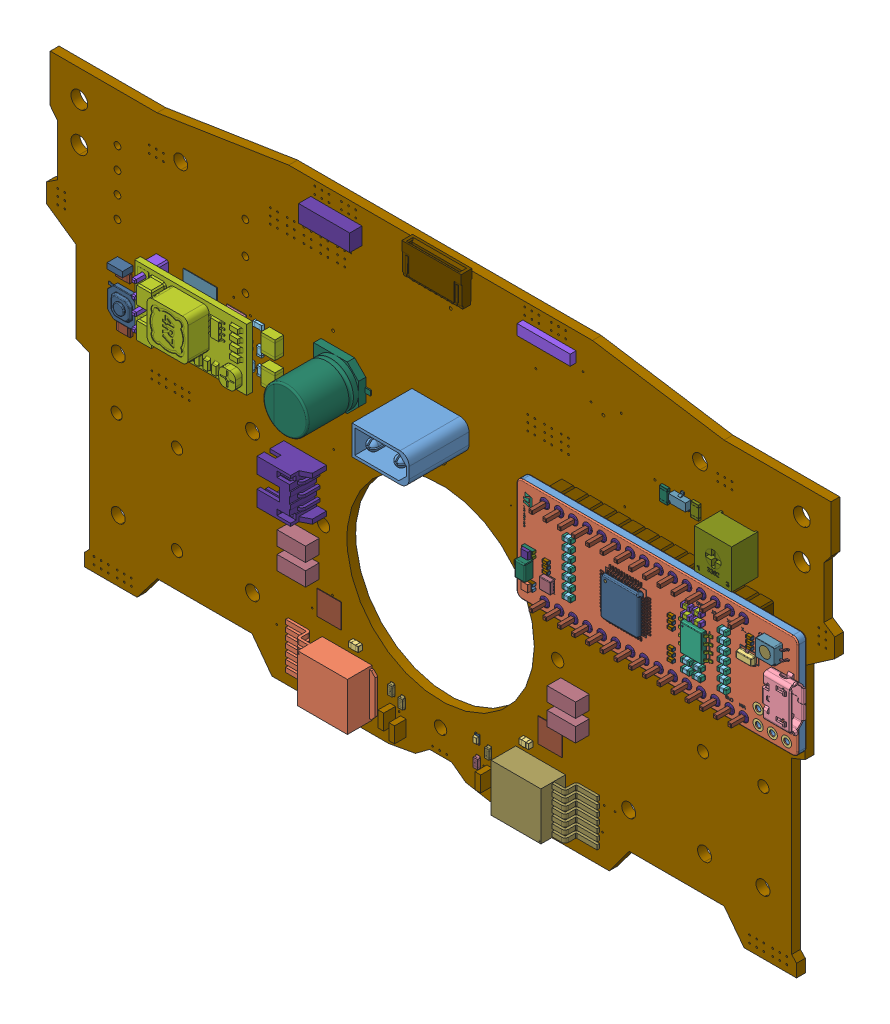
SolidWorks assembly placa v11, configuration Predeterminado. Lengths in mm.
Overall size (140.86 80.97 16.6).
216 component instances, 71 part files, 0 mates.
Components (placement in the parent):
- placa v11.step-1: placa v11.step [Predeterminado] at origin size (140.86 80.97 16.6)
  - PCB Component.step-1: PCB Component.step [Predeterminado] at origin size (140.86 80.97 16.6)
    - LED-0603 (1).step-1: LED-0603 (1).step [Predeterminado] at (70.275 8.61 1.57) x (0 -1 0) z (0 0 1) size (1.61 0.81 0.61)
      - Pocket002.step-1: Pocket002.step [Predeterminado] at origin size (0.41 0.81 0.21)
      - Pad004.step-1: Pad004.step [Predeterminado] x (1 0 0) z (0 0 -1) size (0.4 0.8 0)
      - Fillet.step-1: Fillet.step [Predeterminado] at origin size (1 0.7 0.4)
      - Pocket001.step-1: Pocket001.step [Predeterminado] at origin size (0.4 0.8 0.2)
      - Pad.step-1: Pad.step [Predeterminado] at origin size (0.8 0.8 0.2)
    - ARDUINO-NANO-3.0.step-1: ARDUINO-NANO-3.0.step [Predeterminado] at (104.204 47.47 1.57) size (51.66 18.54 11.82)
      - 1.step.step-1: 1.step.step [Predeterminado] at (9.2423 0.0433 4.14) x (0 -1 0) z (0 0 1) size (4.9 6 1)
        - 1-0.step.step-1: 1-0.step.step [Predeterminado] at (0 0 0.08) size (4.9 3.9 0.92)
        - 2.step.step-1: 2.step.step [Predeterminado] at (0.635 0 0) size (4.23 6 0.62)
        - Name1.step.step-1: Name1.step.step [Predeterminado] at (-0.0045 -0.5756 0.3787) x (-1 0 0) z (0 1 0) size (0.25 0.13 0.25)
        - thermal pad.step.step-1: thermal pad.step.step [Predeterminado] at (0 0 0.08) x (-1 0 0) z (0 0 -1) size (3.2 2.4 0.1)
      - QFP Template.step.step-1: QFP Template.step.step [Predeterminado] at (-3.3256 -0.4727 4.14) x (0 -1 0) z (0 0 1) size (9 9 1.2)
        - Body.step.step-1: Body.step.step [Predeterminado] at (0 0 0.15) size (7 7 1.05)
        - Leg.step.step-1: Leg.step.step [Predeterminado] at (0 0.25 0) x (1 0 0) z (0 -1 0) size (9 0.75 5.72)
        - Leg.step.step-2: Leg.step.step [Predeterminado] at (-0.25 0 0) x (0 1 0) z (1 0 0) size (9 0.75 5.72)
        - name2.step.step-1: name2.step.step [Predeterminado] at (1.2257 1.5908 1.101) size (0.47 0.47 0.1)
      - QFP Template.step (1).step-1: QFP Template.step (1).step [Predeterminado] at (11.7079 0.2587 2.54) x (0 -1 0) z (0 0 -1) size (9 9 1.2)
        - Body.step.step-1: Body.step.step [Predeterminado] at (0 0 0.15) size (7 7 1.05)
        - Leg.step.step-1: Leg.step.step [Predeterminado] at (0 0.25 0) x (1 0 0) z (0 -1 0) size (9 0.75 5.72)
        - Leg.step.step-2: Leg.step.step [Predeterminado] at (-0.25 0 0) x (0 1 0) z (1 0 0) size (9 0.75 5.72)
        - name2.step.step-1: name2.step.step [Predeterminado] at (1.2257 1.5908 1.101) size (0.47 0.47 0.1)
      - 1-1.step.step-1: 1-1.step.step [Predeterminado] at (-17.0798 -4.3486 4.14) size (2 2 0.8)
        - 1-2.step.step-1: 1-2.step.step [Predeterminado] at (0 0 0.02) size (2 2 0.78)
        - 2-3.step.step-1: 2-3.step.step [Predeterminado] at origin size (2 1.6 0.2)
      - 1-2-4.step.step-1: 1-2-4.step.step [Predeterminado] at (-20.4345 -1.0096 4.14) size (2 1.25 1.09)
        - 1-5.step.step-1: 1-5.step.step [Predeterminado] at (0 0 0.01) size (1.98 1.25 0.58)
        - 2-6.step.step-1: 2-6.step.step [Predeterminado] at (0.001 0 0) size (2 1.25 0.6)
        - 3.step.step-1: 3.step.step [Predeterminado] at (0.001 0 0.59) x (-1 0 0) z (0 0 1) size (1.45 1.25 0.5)
      - 1-3.step.step-1: 1-3.step.step [Predeterminado] at (-20.4345 -6.0538 4.14) size (2 1.25 1.09)
        - 1-7.step.step-1: 1-7.step.step [Predeterminado] at (0 0 0.01) size (1.98 1.25 0.58)
        - 2-8.step.step-1: 2-8.step.step [Predeterminado] at (0.001 0 0) size (2 1.25 0.6)
        - 3-9.step.step-1: 3-9.step.step [Predeterminado] at (0.001 0 0.59) x (-1 0 0) z (0 0 1) size (1.45 1.25 0.5)
      - 1-4.step.step-1: 1-4.step.step [Predeterminado] at (18.758 2.4348 4.14) x (0 -1 0) z (0 0 1) size (2.3 2.86 1.1)
        - 1-10.step.step-1: 1-10.step.step [Predeterminado] at (0 0 0.055) size (1.3 2.86 1.04)
        - 2-11.step.step-1: 2-11.step.step [Predeterminado] x (1 0 0) z (0 -1 0) size (2.3 0.55 2.35)
      - 3-12.step.step-1: 3-12.step.step [Predeterminado] at (14.649 -4.6077 5.09) x (-1 0 0) z (0 0 -1) size (1.6 0.8 0.95)
        - 1-13.step.step-1: 1-13.step.step [Predeterminado] at (-0.78 0.38 0.93) x (1 0 0) z (0 0 -1) size (1.56 0.76 0.91)
        - 2-14.step.step-1: 2-14.step.step [Predeterminado] at (0 0 0.95) x (1 0 0) z (0 0 -1) size (1.6 0.8 0.95)
      - 3-12.step (1).step-1: 3-12.step (1).step [Predeterminado] at (-13.1027 -4.224 5.09) x (-1 0 0) z (0 0 -1) size (1.6 0.8 0.95)
        - 1-13.step.step-1: 1-13.step.step [Predeterminado] at (-0.78 0.38 0.93) x (1 0 0) z (0 0 -1) size (1.56 0.76 0.91)
        - 2-14.step.step-1: 2-14.step.step [Predeterminado] at (0 0 0.95) x (1 0 0) z (0 0 -1) size (1.6 0.8 0.95)
      - 3-12.step (2).step-1: 3-12.step (2).step [Predeterminado] at (14.649 -3.1077 5.09) x (-1 0 0) z (0 0 -1) size (1.6 0.8 0.95)
        - 1-13.step.step-1: 1-13.step.step [Predeterminado] at (-0.78 0.38 0.93) x (1 0 0) z (0 0 -1) size (1.56 0.76 0.91)
        - 2-14.step.step-1: 2-14.step.step [Predeterminado] at (0 0 0.95) x (1 0 0) z (0 0 -1) size (1.6 0.8 0.95)
      - 3-12.step (3).step-1: 3-12.step (3).step [Predeterminado] at (-13.1027 -2.724 5.09) x (-1 0 0) z (0 0 -1) size (1.6 0.8 0.95)
        - 1-13.step.step-1: 1-13.step.step [Predeterminado] at (-0.78 0.38 0.93) x (1 0 0) z (0 0 -1) size (1.56 0.76 0.91)
        - 2-14.step.step-1: 2-14.step.step [Predeterminado] at (0 0 0.95) x (1 0 0) z (0 0 -1) size (1.6 0.8 0.95)
      - 3-12.step (4).step-1: 3-12.step (4).step [Predeterminado] at (14.649 -1.6077 5.09) x (-1 0 0) z (0 0 -1) size (1.6 0.8 0.95)
        - 1-13.step.step-1: 1-13.step.step [Predeterminado] at (-0.78 0.38 0.93) x (1 0 0) z (0 0 -1) size (1.56 0.76 0.91)
        - 2-14.step.step-1: 2-14.step.step [Predeterminado] at (0 0 0.95) x (1 0 0) z (0 0 -1) size (1.6 0.8 0.95)
      - 3-12.step (5).step-1: 3-12.step (5).step [Predeterminado] at (-13.1027 -1.224 5.09) x (-1 0 0) z (0 0 -1) size (1.6 0.8 0.95)
        - 1-13.step.step-1: 1-13.step.step [Predeterminado] at (-0.78 0.38 0.93) x (1 0 0) z (0 0 -1) size (1.56 0.76 0.91)
        - 2-14.step.step-1: 2-14.step.step [Predeterminado] at (0 0 0.95) x (1 0 0) z (0 0 -1) size (1.6 0.8 0.95)
      - 3-12.step (6).step-1: 3-12.step (6).step [Predeterminado] at (14.649 -0.1077 5.09) x (-1 0 0) z (0 0 -1) size (1.6 0.8 0.95)
        - 1-13.step.step-1: 1-13.step.step [Predeterminado] at (-0.78 0.38 0.93) x (1 0 0) z (0 0 -1) size (1.56 0.76 0.91)
        - 2-14.step.step-1: 2-14.step.step [Predeterminado] at (0 0 0.95) x (1 0 0) z (0 0 -1) size (1.6 0.8 0.95)
      - 3-12.step (7).step-1: 3-12.step (7).step [Predeterminado] at (-13.1027 0.276 5.09) x (-1 0 0) z (0 0 -1) size (1.6 0.8 0.95)
        - 1-13.step.step-1: 1-13.step.step [Predeterminado] at (-0.78 0.38 0.93) x (1 0 0) z (0 0 -1) size (1.56 0.76 0.91)
        - 2-14.step.step-1: 2-14.step.step [Predeterminado] at (0 0 0.95) x (1 0 0) z (0 0 -1) size (1.6 0.8 0.95)
      - 3-12.step (8).step-1: 3-12.step (8).step [Predeterminado] at (14.649 1.3923 5.09) x (-1 0 0) z (0 0 -1) size (1.6 0.8 0.95)
        - 1-13.step.step-1: 1-13.step.step [Predeterminado] at (-0.78 0.38 0.93) x (1 0 0) z (0 0 -1) size (1.56 0.76 0.91)
        - 2-14.step.step-1: 2-14.step.step [Predeterminado] at (0 0 0.95) x (1 0 0) z (0 0 -1) size (1.6 0.8 0.95)
      - 3-12.step (9).step-1: 3-12.step (9).step [Predeterminado] at (-13.1027 1.776 5.09) x (-1 0 0) z (0 0 -1) size (1.6 0.8 0.95)
        - 1-13.step.step-1: 1-13.step.step [Predeterminado] at (-0.78 0.38 0.93) x (1 0 0) z (0 0 -1) size (1.56 0.76 0.91)
        - 2-14.step.step-1: 2-14.step.step [Predeterminado] at (0 0 0.95) x (1 0 0) z (0 0 -1) size (1.6 0.8 0.95)
      - 3-12.step (10).step-1: 3-12.step (10).step [Predeterminado] at (14.649 2.8923 5.09) x (-1 0 0) z (0 0 -1) size (1.6 0.8 0.95)
        - 1-13.step.step-1: 1-13.step.step [Predeterminado] at (-0.78 0.38 0.93) x (1 0 0) z (0 0 -1) size (1.56 0.76 0.91)
        - 2-14.step.step-1: 2-14.step.step [Predeterminado] at (0 0 0.95) x (1 0 0) z (0 0 -1) size (1.6 0.8 0.95)
      - 3-12.step (11).step-1: 3-12.step (11).step [Predeterminado] at (-13.1027 3.276 5.09) x (-1 0 0) z (0 0 -1) size (1.6 0.8 0.95)
        - 1-13.step.step-1: 1-13.step.step [Predeterminado] at (-0.78 0.38 0.93) x (1 0 0) z (0 0 -1) size (1.56 0.76 0.91)
        - 2-14.step.step-1: 2-14.step.step [Predeterminado] at (0 0 0.95) x (1 0 0) z (0 0 -1) size (1.6 0.8 0.95)
      - 3-12.step (12).step-1: 3-12.step (12).step [Predeterminado] at (14.649 4.3923 5.09) x (-1 0 0) z (0 0 -1) size (1.6 0.8 0.95)
        - 1-13.step.step-1: 1-13.step.step [Predeterminado] at (-0.78 0.38 0.93) x (1 0 0) z (0 0 -1) size (1.56 0.76 0.91)
        - 2-14.step.step-1: 2-14.step.step [Predeterminado] at (0 0 0.95) x (1 0 0) z (0 0 -1) size (1.6 0.8 0.95)
      - 3-12.step (13).step-1: 3-12.step (13).step [Predeterminado] at (-13.1027 4.776 5.09) x (-1 0 0) z (0 0 -1) size (1.6 0.8 0.95)
        - 1-13.step.step-1: 1-13.step.step [Predeterminado] at (-0.78 0.38 0.93) x (1 0 0) z (0 0 -1) size (1.56 0.76 0.91)
        - 2-14.step.step-1: 2-14.step.step [Predeterminado] at (0 0 0.95) x (1 0 0) z (0 0 -1) size (1.6 0.8 0.95)
      - 3-12.step (14).step-1: 3-12.step (14).step [Predeterminado] at (10.1169 -4.9732 4.14) size (1.6 0.8 0.95)
        - 1-13.step.step-1: 1-13.step.step [Predeterminado] at (-0.78 0.38 0.93) x (1 0 0) z (0 0 -1) size (1.56 0.76 0.91)
        - 2-14.step.step-1: 2-14.step.step [Predeterminado] at (0 0 0.95) x (1 0 0) z (0 0 -1) size (1.6 0.8 0.95)
      - 3-12.step (15).step-1: 3-12.step (15).step [Predeterminado] at (8.1169 -4.9732 4.14) size (1.6 0.8 0.95)
        - 1-13.step.step-1: 1-13.step.step [Predeterminado] at (-0.78 0.38 0.93) x (1 0 0) z (0 0 -1) size (1.56 0.76 0.91)
        - 2-14.step.step-1: 2-14.step.step [Predeterminado] at (0 0 0.95) x (1 0 0) z (0 0 -1) size (1.6 0.8 0.95)
      - 3-12.step (16).step-1: 3-12.step (16).step [Predeterminado] at (10.1169 -3.4732 4.14) size (1.6 0.8 0.95)
        - 1-13.step.step-1: 1-13.step.step [Predeterminado] at (-0.78 0.38 0.93) x (1 0 0) z (0 0 -1) size (1.56 0.76 0.91)
        - 2-14.step.step-1: 2-14.step.step [Predeterminado] at (0 0 0.95) x (1 0 0) z (0 0 -1) size (1.6 0.8 0.95)
      - 3-12.step (17).step-1: 3-12.step (17).step [Predeterminado] at (8.1169 -3.4732 4.14) size (1.6 0.8 0.95)
        - 1-13.step.step-1: 1-13.step.step [Predeterminado] at (-0.78 0.38 0.93) x (1 0 0) z (0 0 -1) size (1.56 0.76 0.91)
        - 2-14.step.step-1: 2-14.step.step [Predeterminado] at (0 0 0.95) x (1 0 0) z (0 0 -1) size (1.6 0.8 0.95)
      - 3_MIR.step.step-1: 3_MIR.step.step [Predeterminado] at (10.1169 4.9732 4.14) x (1 0 0) z (0 0 -1) size (1.6 0.8 0.95)
        - 1_MIR.step.step-1: 1_MIR.step.step [Predeterminado] at (-0.78 0.38 -0.93) x (1 0 0) z (0 0 -1) size (1.56 0.76 0.91)
        - 2_MIR.step.step-1: 2_MIR.step.step [Predeterminado] at (0 0 -0.95) x (1 0 0) z (0 0 -1) size (1.6 0.8 0.95)
      - 3_MIR.step (1).step-1: 3_MIR.step (1).step [Predeterminado] at (8.1169 4.9732 4.14) x (1 0 0) z (0 0 -1) size (1.6 0.8 0.95)
        - 1_MIR.step.step-1: 1_MIR.step.step [Predeterminado] at (-0.78 0.38 -0.93) x (1 0 0) z (0 0 -1) size (1.56 0.76 0.91)
        - 2_MIR.step.step-1: 2_MIR.step.step [Predeterminado] at (0 0 -0.95) x (1 0 0) z (0 0 -1) size (1.6 0.8 0.95)
      - 3_MIR.step (2).step-1: 3_MIR.step (2).step [Predeterminado] at (10.1169 3.4732 4.14) x (1 0 0) z (0 0 -1) size (1.6 0.8 0.95)
        - 1_MIR.step.step-1: 1_MIR.step.step [Predeterminado] at (-0.78 0.38 -0.93) x (1 0 0) z (0 0 -1) size (1.56 0.76 0.91)
        - 2_MIR.step.step-1: 2_MIR.step.step [Predeterminado] at (0 0 -0.95) x (1 0 0) z (0 0 -1) size (1.6 0.8 0.95)
      - 3_MIR.step (3).step-1: 3_MIR.step (3).step [Predeterminado] at (8.1169 3.4732 4.14) x (1 0 0) z (0 0 -1) size (1.6 0.8 0.95)
        - 1_MIR.step.step-1: 1_MIR.step.step [Predeterminado] at (-0.78 0.38 -0.93) x (1 0 0) z (0 0 -1) size (1.56 0.76 0.91)
        - 2_MIR.step.step-1: 2_MIR.step.step [Predeterminado] at (0 0 -0.95) x (1 0 0) z (0 0 -1) size (1.6 0.8 0.95)
      - 3-1.step.step-1: 3-1.step.step [Predeterminado] at (19.0751 5.5632 4.69) x (-1 0 0) z (0 0 -1) size (1 0.5 0.55)
        - 1-15.step.step-1: 1-15.step.step [Predeterminado] at (-0.49 0.24 0.54) x (1 0 0) z (0 0 -1) size (0.98 0.48 0.53)
        - 2-16.step.step-1: 2-16.step.step [Predeterminado] at (-0.5 0.25 0.55) x (1 0 0) z (0 0 -1) size (1 0.5 0.55)
      - 3-1.step (1).step-1: 3-1.step (1).step [Predeterminado] at (19.0751 4.7491 4.69) x (-1 0 0) z (0 0 -1) size (1 0.5 0.55)
        - 1-15.step.step-1: 1-15.step.step [Predeterminado] at (-0.49 0.24 0.54) x (1 0 0) z (0 0 -1) size (0.98 0.48 0.53)
        - 2-16.step.step-1: 2-16.step.step [Predeterminado] at (-0.5 0.25 0.55) x (1 0 0) z (0 0 -1) size (1 0.5 0.55)
      - 3-1.step (2).step-1: 3-1.step (2).step [Predeterminado] at (19.0751 3.9392 4.69) x (-1 0 0) z (0 0 -1) size (1 0.5 0.55)
        - 1-15.step.step-1: 1-15.step.step [Predeterminado] at (-0.49 0.24 0.54) x (1 0 0) z (0 0 -1) size (0.98 0.48 0.53)
        - 2-16.step.step-1: 2-16.step.step [Predeterminado] at (-0.5 0.25 0.55) x (1 0 0) z (0 0 -1) size (1 0.5 0.55)
      - 3-1.step (3).step-1: 3-1.step (3).step [Predeterminado] at (-17.3312 -0.9835 4.69) x (-1 0 0) z (0 0 -1) size (1 0.5 0.55)
        - 1-15.step.step-1: 1-15.step.step [Predeterminado] at (-0.49 0.24 0.54) x (1 0 0) z (0 0 -1) size (0.98 0.48 0.53)
        - 2-16.step.step-1: 2-16.step.step [Predeterminado] at (-0.5 0.25 0.55) x (1 0 0) z (0 0 -1) size (1 0.5 0.55)
      - 3-1.step (4).step-1: 3-1.step (4).step [Predeterminado] at (-17.3312 -2.5605 4.69) x (-1 0 0) z (0 0 -1) size (1 0.5 0.55)
        - 1-15.step.step-1: 1-15.step.step [Predeterminado] at (-0.49 0.24 0.54) x (1 0 0) z (0 0 -1) size (0.98 0.48 0.53)
        - 2-16.step.step-1: 2-16.step.step [Predeterminado] at (-0.5 0.25 0.55) x (1 0 0) z (0 0 -1) size (1 0.5 0.55)
      - 3-1.step (5).step-1: 3-1.step (5).step [Predeterminado] at (-17.3312 -1.7295 4.69) x (-1 0 0) z (0 0 -1) size (1 0.5 0.55)
        - 1-15.step.step-1: 1-15.step.step [Predeterminado] at (-0.49 0.24 0.54) x (1 0 0) z (0 0 -1) size (0.98 0.48 0.53)
        - 2-16.step.step-1: 2-16.step.step [Predeterminado] at (-0.5 0.25 0.55) x (1 0 0) z (0 0 -1) size (1 0.5 0.55)
      - 3-1.step (6).step-1: 3-1.step (6).step [Predeterminado] at (5.0242 -5.0165 4.69) x (-1 0 0) z (0 0 -1) size (1 0.5 0.55)
        - 1-15.step.step-1: 1-15.step.step [Predeterminado] at (-0.49 0.24 0.54) x (1 0 0) z (0 0 -1) size (0.98 0.48 0.53)
        - 2-16.step.step-1: 2-16.step.step [Predeterminado] at (-0.5 0.25 0.55) x (1 0 0) z (0 0 -1) size (1 0.5 0.55)
      - 3-1.step (7).step-1: 3-1.step (7).step [Predeterminado] at (5.0242 -4.0978 4.69) x (-1 0 0) z (0 0 -1) size (1 0.5 0.55)
        - 1-15.step.step-1: 1-15.step.step [Predeterminado] at (-0.49 0.24 0.54) x (1 0 0) z (0 0 -1) size (0.98 0.48 0.53)
        - 2-16.step.step-1: 2-16.step.step [Predeterminado] at (-0.5 0.25 0.55) x (1 0 0) z (0 0 -1) size (1 0.5 0.55)
      - 3-1.step (8).step-1: 3-1.step (8).step [Predeterminado] at (5.0242 -3.2174 4.69) x (-1 0 0) z (0 0 -1) size (1 0.5 0.55)
        - 1-15.step.step-1: 1-15.step.step [Predeterminado] at (-0.49 0.24 0.54) x (1 0 0) z (0 0 -1) size (0.98 0.48 0.53)
        - 2-16.step.step-1: 2-16.step.step [Predeterminado] at (-0.5 0.25 0.55) x (1 0 0) z (0 0 -1) size (1 0.5 0.55)
      - 3-1.step (9).step-1: 3-1.step (9).step [Predeterminado] at (5.0242 -0.0165 4.69) x (-1 0 0) z (0 0 -1) size (1 0.5 0.55)
        - 1-15.step.step-1: 1-15.step.step [Predeterminado] at (-0.49 0.24 0.54) x (1 0 0) z (0 0 -1) size (0.98 0.48 0.53)
        - 2-16.step.step-1: 2-16.step.step [Predeterminado] at (-0.5 0.25 0.55) x (1 0 0) z (0 0 -1) size (1 0.5 0.55)
      - 3-1.step (10).step-1: 3-1.step (10).step [Predeterminado] at (5.0242 0.9022 4.69) x (-1 0 0) z (0 0 -1) size (1 0.5 0.55)
        - 1-15.step.step-1: 1-15.step.step [Predeterminado] at (-0.49 0.24 0.54) x (1 0 0) z (0 0 -1) size (0.98 0.48 0.53)
        - 2-16.step.step-1: 2-16.step.step [Predeterminado] at (-0.5 0.25 0.55) x (1 0 0) z (0 0 -1) size (1 0.5 0.55)
      - 3-1.step (11).step-1: 3-1.step (11).step [Predeterminado] at (5.0242 1.7826 4.69) x (-1 0 0) z (0 0 -1) size (1 0.5 0.55)
        - 1-15.step.step-1: 1-15.step.step [Predeterminado] at (-0.49 0.24 0.54) x (1 0 0) z (0 0 -1) size (0.98 0.48 0.53)
        - 2-16.step.step-1: 2-16.step.step [Predeterminado] at (-0.5 0.25 0.55) x (1 0 0) z (0 0 -1) size (1 0.5 0.55)
      - 1-17.step.step-1: 1-17.step.step [Predeterminado] at (2.2426 0 2.54) x (0 -1 0) z (0 0 1) size (15.88 36.2 11.76)
      - 2-18.step.step-1: 2-18.step.step [Predeterminado] at (2.2426 0 2.54) x (0 -1 0) z (0 0 1) size (1.95 1.95 0.2)
      - 3-19.step.step-1: 3-19.step.step [Predeterminado] at (2.2426 0 2.54) x (0 -1 0) z (0 0 1) size (1.8 5.28 0.86)
      - 4.step.step-1: 4.step.step [Predeterminado] at (2.2426 0 2.54) x (0 -1 0) z (0 0 1) size (2.98 3.39 1.49)
      - 6.step.step-1: 6.step.step [Predeterminado] at (2.2426 0 2.54) x (0 -1 0) z (0 0 1) size (2.83 1.84 1.5)
      - 7.step.step-1: 7.step.step [Predeterminado] at (2.2426 0 2.54) x (0 -1 0) z (0 0 1) size (0.97 0.6 0.51)
      - 8.step.step-1: 8.step.step [Predeterminado] at (2.2426 0 2.54) x (0 -1 0) z (0 0 1) size (16.96 37.28 0.1)
      - 9.step.step-1: 9.step.step [Predeterminado] at (2.2426 0 2.54) x (0 -1 0) z (0 0 1) size (17.78 38.1 2.54)
      - 10.step.step-1: 10.step.step [Predeterminado] at (2.2426 0 2.54) x (0 -1 0) z (0 0 1) size (18.54 50.29 1.2)
      - 11.step.step-1: 11.step.step [Predeterminado] at (2.2426 0 2.54) x (0 -1 0) z (0 0 1) size (18.54 50.29 1.6)
      - 12.step.step-1: 12.step.step [Predeterminado] at (2.2426 0 2.54) x (0 -1 0) z (0 0 1) size (4.34 6.88 1.6)
      - USB Connector.step.step-1: USB Connector.step.step [Predeterminado] at (26.0074 -0.1867 5.365) x (0 1 0) z (1 0 0) size (8.2 3.3 5.4)
      - 13.step.step-1: 13.step.step [Predeterminado] at (2.2426 0 4.14) x (0 -1 0) z (0 0 1) size (12.46 38.74 0)
      - STM Logo.step.step-1: STM Logo.step.step [Predeterminado] at (-19.8495 -2.5718 4.041) x (0 -1 0) z (0 0 1) size (5.5 1.52 0.1)
    - HW-613.step-1: HW-613.step [Predeterminado] at (12.49 44.591 1.57) size (20 11 13.1)
      - 05KJ_Mini_PCB_Regulator.step-1: 05KJ_Mini_PCB_Regulator.step [Predeterminado] at (19.8629 10.8309 2.3992) x (0 -1 0) z (-1 0 0) size (11 4.81 20)
      - 1_Male_Pin_2.54_mm.step-1: 1_Male_Pin_2.54_mm.step [Predeterminado] at (1.6879 8.8159 5.3992) x (0 1 0) z (-1 0 0) size (2.54 11.1 2.4)
      - 1_Male_Pin_2.54_mm.step-2: 1_Male_Pin_2.54_mm.step [Predeterminado] at (1.6879 6.2759 5.3992) x (0 1 0) z (-1 0 0) size (2.54 11.1 2.4)
      - 1_Male_Pin_2.54_mm.step-3: 1_Male_Pin_2.54_mm.step [Predeterminado] at (1.6879 3.7359 5.3992) x (0 1 0) z (-1 0 0) size (2.54 11.1 2.4)
      - 1_Male_Pin_2.54_mm.step-4: 1_Male_Pin_2.54_mm.step [Predeterminado] at (1.6879 1.1959 5.3992) x (0 1 0) z (-1 0 0) size (2.54 11.1 2.4)
    - Board.step-1: Board.step [Predeterminado] at origin size (140.86 80.59 1.57)
    - MOMENTARY-SWITCH-SPST-SMD-5.2-REDUNDANT.step-1: MOMENTARY-SWITCH-SPST-SMD-5.2-REDUNDANT.step [Predeterminado] at (7.486 44.336 1.57) size (6.4 5.3 1.5)
    - 10k_2.step-1: 10k_2.step [Predeterminado] at (7.386 40.707 1.57) size (2.5 1.4 0.5)
    - LED-0603.step-1: LED-0603.step [Predeterminado] at (55.035 8.61 1.57) x (0 -1 0) z (0 0 1) size (2.1 0.8 0.6)
    - 10k.step-1: 10k.step [Predeterminado] at (70.312 4.989 1.57) x (0 -1 0) z (0 0 1) size (2.1 0.8 0.6)
    - 2N7002CK.step-1: 2N7002CK.step [Predeterminado] at (106.952 63.962 1.57) size (3 2.5 1.1)
    - 103.step-1: 103.step [Predeterminado] at (103.896 63.305 1.57) x (0 -1 0) z (0 0 1) size (2.5 1.4 0.5)
    - 10k_1.step-1: 10k_1.step [Predeterminado] at (109.485 63.628 1.57) x (0 -1 0) z (0 0 1) size (2.5 1.4 0.5)
    - JST-XH-03-PIN-LONG-PAD.step-1: JST-XH-03-PIN-LONG-PAD.step [Predeterminado] at (39.428 34.17 1.57) x (0 -1 0) z (0 0 1) size (7.9 7.6 8.2)
    - FH12-08S-1SH.step-1: FH12-08S-1SH.step [Predeterminado] at (63.91 77.561 1.57) x (-1 0 0) z (0 0 1) size (10.6 6.5 1.92)
    - 10k_2.step-2: 10k_2.step [Predeterminado] at (7.262 48.989 1.57) size (2.5 1.4 0.5)
    - LED-0603.step-2: LED-0603.step [Predeterminado] at (56.895 7.53 1.57) x (0 -1 0) z (0 0 1) size (2.1 0.8 0.6)
    - LED-0603.step-3: LED-0603.step [Predeterminado] at (72.322 7.486 1.57) x (0 -1 0) z (0 0 1) size (2.1 0.8 0.6)
    - XT30UPB-M.step-1: XT30UPB-M.step [Predeterminado] at (63.686 54.256 1.57) x (-1 0 0) z (0 0 1) size (10.2 5.25 13.7)
    - TLE5206-2G.step-1: TLE5206-2G.step [Predeterminado] at (44.309 6.214 1.57) x (0 -1 0) z (0 0 1) size (8.52 16 4.4)
    - CAPC1608X85.step-1: CAPC1608X85.step [Predeterminado] at (79.287 12.679 1.57) x (-1 0 0) z (0 0 1) size (1.75 0.95 0.85)
    - CAPC1608X85.step-2: CAPC1608X85.step [Predeterminado] at (48.839 12.459 1.57) x (-1 0 0) z (0 0 1) size (1.75 0.95 0.85)
    - MP2315GJ.step-1: MP2315GJ.step [Predeterminado] at (26.969 52.158 1.57) x (-1 0 0) z (0 0 1) size (3.46 2.1 0.1)
    - 200k.step-1: 200k.step [Predeterminado] at (27.103 47.618 1.57) size (1.6 0.86 0.51)
    - 200k.step-2: 200k.step [Predeterminado] at (29.997 46.286 1.57) x (0 1 0) z (0 0 1) size (1.6 0.86 0.51)
    - 200k.step-3: 200k.step [Predeterminado] at (24.743 45.644 1.57) size (1.6 0.86 0.51)
    - 200k.step-4: 200k.step [Predeterminado] at (31.702 46.341 1.57) x (0 -1 0) z (0 0 1) size (1.6 0.86 0.51)
    - 200k.step-5: 200k.step [Predeterminado] at (31.645 49.39 1.57) x (0 1 0) z (0 0 1) size (1.6 0.86 0.51)
    - 200k.step-6: 200k.step [Predeterminado] at (31.3 53.202 1.57) size (1.6 0.86 0.51)
    - 22uf.step-1: 22uf.step [Predeterminado] at (23.406 47.636 1.57) size (1.6 0.86 0.86)
    - 22uf.step-2: 22uf.step [Predeterminado] at (27.652 45.634 1.57) size (1.6 0.86 0.86)
    - 22uf.step-3: 22uf.step [Predeterminado] at (18.728 45.514 1.57) size (1.6 0.86 0.86)
    - 22uf.step-4: 22uf.step [Predeterminado] at (21.82 45.634 1.57) x (-1 0 0) z (0 0 1) size (1.6 0.86 0.86)
    - 22uf.step-5: 22uf.step [Predeterminado] at (29.634 49.37 1.57) x (0 1 0) z (0 0 1) size (1.6 0.86 0.86)
    - 22uf.step-6: 22uf.step [Predeterminado] at (18.755 47.622 1.57) size (1.6 0.86 0.86)
    - C1210.step-1: C1210.step [Predeterminado] at (34.29 52.07 1.57) x (0 -1 0) z (0 0 1) size (3.2 2.5 1.55)
    - C1210.step-2: C1210.step [Predeterminado] at (34.29 46.99 1.57) x (0 1 0) z (0 0 1) size (3.2 2.5 1.55)
    - 1X04.step-1: 1X04.step [Predeterminado] at (79.26 76.438 1.57) size (9.5 1.88 1.05)
    - 10k_3.step-1: 10k_3.step [Predeterminado] at (55.035 4.8 1.57) x (0 -1 0) z (0 0 1) size (2.8 1 2.1)
    - 10k_3.step-2: 10k_3.step [Predeterminado] at (92.194 65.647 0) x (0 1 0) z (0 0 -1) size (2.8 1 2.1)
    - 10k_3.step-3: 10k_3.step [Predeterminado] at (35.601 12.641 0) x (0 -1 0) z (0 0 -1) size (2.8 1 2.1)
    - 10k_3.step-4: 10k_3.step [Predeterminado] at (47.48 65.436 0) x (0 1 0) z (0 0 -1) size (2.8 1 2.1)
    - 10k_3.step-5: 10k_3.step [Predeterminado] at (82.596 12.429 0) x (0 -1 0) z (0 0 -1) size (2.8 1 2.1)
    - 10k_3.step-6: 10k_3.step [Predeterminado] at (56.965 3.798 1.57) x (0 1 0) z (0 0 1) size (2.8 1 2.1)
    - 10k_3.step-7: 10k_3.step [Predeterminado] at (72.365 3.894 1.57) x (0 -1 0) z (0 0 1) size (2.8 1 2.1)
    - LED-0603 (2).step-1: LED-0603 (2).step [Predeterminado] at (86.133 65.321 0) x (1 0 0) z (0 0 -1) size (2.75 1 1.86)
    - LED-0603 (2).step-2: LED-0603 (2).step [Predeterminado] at (41.633 11.485 0) x (1 0 0) z (0 0 -1) size (2.75 1 1.86)
    - LED-0603 (2).step-3: LED-0603 (2).step [Predeterminado] at (41.68 65.48 0) x (1 0 0) z (0 0 -1) size (2.75 1 1.86)
    - LED-0603 (2).step-4: LED-0603 (2).step [Predeterminado] at (85.968 11.242 0) x (1 0 0) z (0 0 -1) size (2.75 1 1.86)
    - LED-0603 (2).step-5: LED-0603 (2).step [Predeterminado] at (7.24 50.476 1.57) size (2.75 1 1.86)
    - 153CLV-0405.step-1: 153CLV-0405.step [Predeterminado] at (43.742 15.388 1.57) x (-1 0 0) z (0 0 1) size (4.3 4.3 0.1)
    - 153CLV-0405.step-2: 153CLV-0405.step [Predeterminado] at (83.228 15.388 1.57) x (-1 0 0) z (0 0 1) size (4.3 4.3 0.1)
    - TLE5206-2G_1.step-1: TLE5206-2G_1.step [Predeterminado] at (84.077 6.486 1.57) x (0 1 0) z (0 0 1) size (8.52 16 4.4)
    - SMD2,54-5,08.step-1: SMD2,54-5,08.step [Predeterminado] at (39.37 24.13 1.57) x (0 1 0) z (0 0 1) size (2.54 5.08 2.44)
    - SMD2,54-5,08.step-2: SMD2,54-5,08.step [Predeterminado] at (39.37 20.32 1.57) x (0 1 0) z (0 0 1) size (2.54 5.08 2.44)
    - SMD2,54-5,08.step-3: SMD2,54-5,08.step [Predeterminado] at (87.63 24.13 1.57) x (0 1 0) z (0 0 1) size (2.54 5.08 2.44)
    - SMD2,54-5,08.step-4: SMD2,54-5,08.step [Predeterminado] at (87.63 20.32 1.57) x (0 1 0) z (0 0 1) size (2.54 5.08 2.44)
    - 4.2uh.step-1: 4.2uh.step [Predeterminado] at (20.701 52.121 1.57) x (-1 0 0) z (0 0 1) size (6 6 0.1)
    - 153CLV-0807.step-1: 153CLV-0807.step [Predeterminado] at (46.349 52.61 1.57) size (9.8 8 10.51)
    - B25P.step-1: B25P.step [Predeterminado] at (117 62 1.57) size (6.61 7.21 6.73)
    - MA04-1.step-1: MA04-1.step [Predeterminado] at (44.979 76.037 1.57) size (9.14 3.05 2.19)
